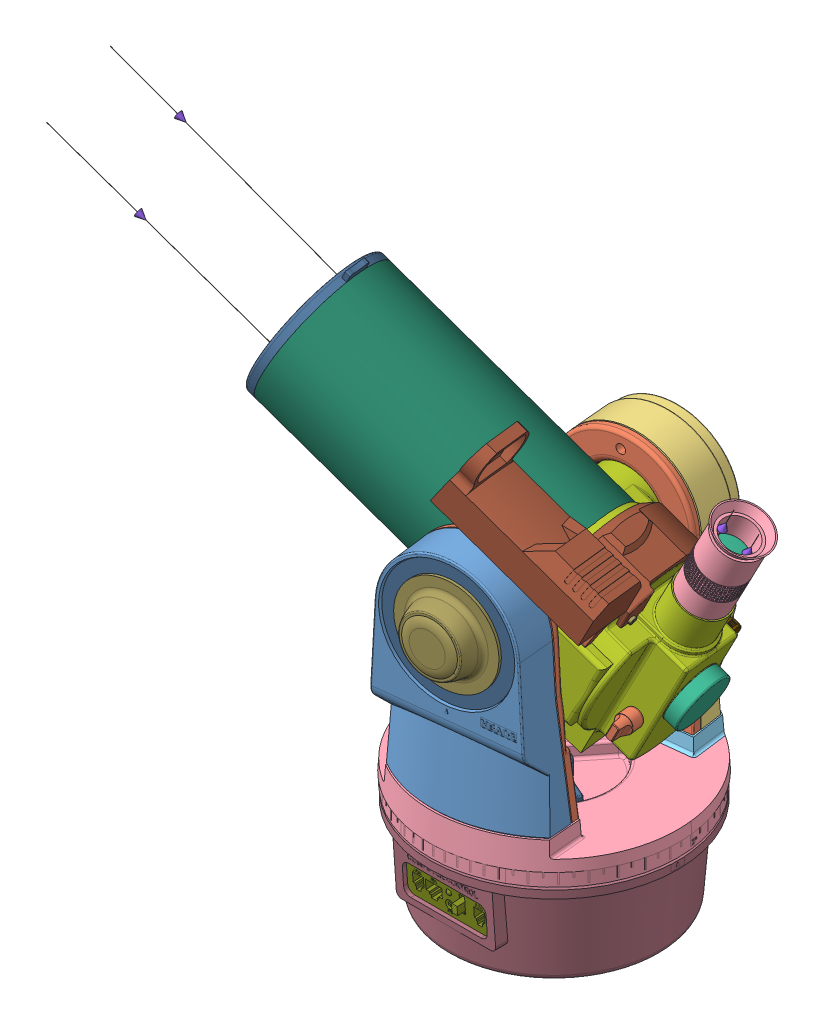
SolidWorks assembly meade, configuration Défaut. Lengths in mm.
Overall size (480.47 493.64 231.58).
168 component instances, 89 part files, 11 mates.
Components (placement in the parent):
- fourche-1: fourche [Défaut] at (-637.6539 13.0791 484.13) x (0.045417 -0.017413 0.998816) z (-0.998966 0.001172 0.045444) size (198.85 238.33 188.61)
  - branche equilibrage-1: branche equilibrage [Défaut] at (-444.0293 45.9192 -837.0232) x (0.999848 0.017413 0.00001) z (0.00001 -0.001172 0.999999) size (42.16 177.75 110.07)
  - Plaque carter équilibrage-1: Plaque carter équilibrage [Défaut] at (-443.0317 45.9366 -837.0903) x (0.999848 0.017413 0.00001) z (0.00001 -0.001172 0.999999) size (27.56 165.18 109.18)
  - Plaque carter équilibrage-2: Plaque carter équilibrage [Défaut] at (-468.0617 45.0668 -480.7137) x (-0.999848 -0.017413 -0.00001) z (-0.00001 0.001172 -0.999999) size (27.56 165.18 109.18)
  - branche motorisée-1: branche motorisée [Défaut] at (-441.716 45.9434 -837.1795) x (0.999848 0.017413 0.00001) z (0.00001 -0.001172 0.999999) size (49.59 177.72 110.04)
  - PIED DE fourche-1: PIED DE fourche [Défaut] at (-454.4692 -14.4541 -658.8869) x (0.999848 0.017413 0.00001) z (0.00001 -0.001172 0.999999) size (191.94 35.1 188.57)
    - Pied de fourche-1: Pied de fourche [Défaut] at (12.1809 59.9857 -178.2534) size (191.94 35.1 188.57)
    - Pied de fourche1-1: Pied de fourche1 [Défaut] at (-12.1809 59.9857 178.0188) x (-1 0 0) z (0 0 -1) size (54.8 35.1 115.86)
  - rondelle vis m8_50-1: rondelle vis m8_50 [Défaut] at (-454.2843 -25.0712 -659.0167) x (0.997592 0.017452 -0.067129) z (0.017413 -0.999848 -0.001172) size (26.8 26.16 7)
  - VisHM8_50-1: VisHM8_50 [Défaut] at (-454.3818 -19.4721 -659.0102) x (0.997592 0.017452 -0.067129) z (0.017413 -0.999848 -0.001172) size (12.6 14.55 55.47)
  - limiteur de couple embase-1: limiteur de couple embase [Défaut] at (-453.5008 -70.0544 -659.0694) x (0.06714 0 0.997744) z (-0.997592 -0.017452 0.067129) size (25.3 5 25.3)
  - Roue à denture hélicoïdale m=0,5 Z=60-1: Roue à denture hélicoïdale m=0,5 Z=60 [Défaut] at (-453.6431 -61.8856 -659.0599) x (0.201032 0.002353 0.979582) z (-0.017413 0.999848 0.001172) size (31.07 31.07 6.34)
  - Levier de débrayage-1: Levier de débrayage [Défaut] at (-491.4971 43.1006 -833.8173) x (0.963244 0.01709 -0.268082) z (0.268062 0.003539 0.963395) size (36.12 10 38.96)
  - plateau-1: plateau [Défaut] at (-454.3861 -19.2221 -659.0099) x (-0.997592 -0.017452 0.067129) z (0.017413 -0.999848 -0.001172) size (170 170 47)
  - EcrouHM 20-2: EcrouHM 20 [Défaut] at (-453.9456 -44.5183 -659.0395) x (0.06714 0 0.997744) z (-0.017413 0.999848 0.001172) size (30 34.64 12)
  - motoreducteur fourche-1: motoreducteur fourche [Défaut] at (-542.1299 45.8782 -641.824) x (0.06714 0 0.997744) z (0.997592 0.017452 -0.067129) size (70.5 139.71 33.06)
    - rep. 01 pignon arbre moteur + disque-1: rep. 01 pignon arbre moteur + disque [Défaut] at (0 -0.36 0) size (19 10.8 19)
    - rep. 02-03 roue Z56-1: rep. 02-03 roue Z56 [Défaut] at (0.8779 -0.6486 0.8082) x (0.995701 0 0.092628) z (-0.092628 0 0.995701) size (28.76 10.95 28.76)
    - rep. 08-09 roue inter-1: rep. 08-09 roue inter [Défaut] at (-0.15 -0.2381 0) x (1 0 0) z (0 0 1) size (12.96 5.74 12.96)
    - rep. 06-07 roue inter-1: rep. 06-07 roue inter [Défaut] at (-0.15 -0.0981 0) x (1 0 0) z (0 0 1) size (13 5.74 13)
    - rep. 04-05 roue inter-1: rep. 04-05 roue inter [Défaut] at (-21.6079 -0.6386 5.1059) x (0.907401 0 -0.420265) z (0.420265 0 0.907401) size (13 5.74 13)
    - bati-1: bati [Défaut] at (103.3128 129.885 -87.3106) size (70.5 138.91 24)
      - Axe Rep19bis-1: Axe Rep19bis [Défaut] at (-92.1856 -130.245 98.2871) x (-0.137137 0 0.990552) z (-0.990552 0 -0.137137) size (3 14 3)
      - moteur-1: moteur [Défaut] at (-103.3128 -129.885 87.3106) size (18 46.5 24)
      - axe-1: axe [Défaut] at (-111.605 -120.0821 97.7106) x (0.934599 0 -0.355704) z (0 -1 0) size (3 3 39)
      - bati2-1: bati2 [Défaut] at (-77.4849 -277.8736 138.6581) x (1 0 0) z (0 0 -1) size (17.4 55.11 17.4)
        - rondelle alu-1: rondelle alu [Défaut] at (-55.9783 -35.2009 30.6529) size (17.4 2.5 17.4)
        - Rondelle M6_1-1: Rondelle M6_1 [Défaut] at (-55.9783 -35.2009 30.6529) size (16.67 2.55 16.67)
        - rondelle alu_1-1: rondelle alu_1 [Défaut] at (-55.9783 -35.2009 30.6529) size (17.4 2.5 17.4)
        - Entretoise_1-1: Entretoise_1 [Défaut] at (-55.9783 -35.2009 30.6529) size (16.5 6 16.5)
        - Entretoise-1: Entretoise [Défaut] at (-55.9783 -35.2009 30.6529) size (16.5 6 16.5)
        - Rondelle M6-1: Rondelle M6 [Défaut] at (-55.9783 -35.2009 30.6529) size (16.67 2.55 16.67)
        - rep. 16 Ecrou M6-1: rep. 16 Ecrou M6 [Défaut] at (18.5294 -120.4752 48.0628) x (-0.896454 0 -0.443136) z (-0.443136 0 0.896454) size (12.68 6 11.39)
      - corps1-1: corps1 [Défaut] at (-126.5989 -147.7633 97.7106) size (62.7 74.5 12)
      - corps2-1: corps2 [Défaut] at (-126.5989 -147.7633 85.7106) size (62.7 50 12) (hidden)
      - châpe en alu-1: châpe en alu [Défaut] at (-133.4632 -157.3984 87.2051) size (33.3 38 19.61)
    - vis-1: vis [Défaut] at (7.3554 -71.4832 9.6533) x (1 0 0) z (0 1 0) size (33.09 33.06 82.71)
      - Vis san fin m=0,5 - 1 filet(s)-2: Vis san fin m=0,5 - 1 filet(s) [Défaut] at (-0.6479 -0.6412 0.3804) x (0.7262 -0.687484 0) z (0 0 1) size (8.16 8.16 68.9)
      - rep12-4: rep12 [Défaut] at (-11.6724 36.0347 43.7266) x (0.537117 -0.843508 0) z (-0.843508 -0.537117 0) size (23.91 29.81 24)
    - engrenage-1: engrenage [Défaut] at (-45.9983 -125.8694 31.0757) x (-0.919401 0 0.393321) z (0.393321 0 0.919401) size (12.99 17.44 12.99)
      - rep.11SLDPRT-1: rep.11SLDPRT [Défaut] at (-64.557 -106.8565 -14.5787) size (9.52 16 9.52)
      - rep. yacine-1: rep. yacine [Défaut] at (-64.557 -106.8565 -14.5787) size (12.99 1.44 12.99)
    - Vis à tête cylindrique à six pans creux Chc M2,5 - 8-1: Vis à tête cylindrique à six pans creux Chc M2,5 - 8 [Défaut] at (6.7074 -20.6971 10.2945) x (0.636786 0 0.771041) z (0 -1 0) size (4.2 4.2 10.57)
    - joint 9 5 emb-1: joint 9 5 emb [Défaut] at (6.7074 -89.1506 10.2945) size (13.5 2 13.5)
    - joint 9 5 emb-2: joint 9 5 emb [Défaut] at (6.7074 -53.1506 10.2945) size (13.5 2 13.5)
  - Vis sans tête à six pans creux à bout cuvette M3 - 3-1: Vis sans tête à six pans creux à bout cuvette M3 - 3 [Réaliste] at (-445.1418 -17.1499 -659.6319) x (-0.019293 -0.859815 -0.51024) z (0.066624 -0.510307 0.857408) size (3.03 3.08 3.04)
  - Vis à tête cylindrique bombée cruciforme type H M3 - 10-1: Vis à tête cylindrique bombée cruciforme type H M3 - 10 [Filetage Réaliste] at (-521.841 56.7793 -695.504) x (-0.997592 -0.017452 0.067129) z (-0.0364 0.955572 -0.292501) size (12.58 5.6 5.6)
  - Vis à tête cylindrique bombée cruciforme type H M3 - 10-2: Vis à tête cylindrique bombée cruciforme type H M3 - 10 [Filetage Réaliste] at (-508.9533 16.8988 -611.179) x (-0.997592 -0.017452 0.067129) z (-0.040277 -0.642181 -0.765494) size (12.58 5.6 5.6)
  - Vis à tête cylindrique bombée cruciforme type H M3 - 10-3: Vis à tête cylindrique bombée cruciforme type H M3 - 10 [Filetage Réaliste] at (-514.8616 16.8988 -698.9804) x (-0.997592 -0.017452 0.067129) z (-0.068087 0.06176 -0.995766) size (12.58 5.6 5.6)
  - Vis à tête cylindrique bombée cruciforme type H M3 - 10-4: Vis à tête cylindrique bombée cruciforme type H M3 - 10 [Filetage Réaliste] at (-521.2936 154.7556 -654.4481) x (-0.997592 -0.017452 0.067129) z (-0.06714 0 -0.997744) size (12.58 5.6 5.6)
  - Vis à tête cylindrique bombée cruciforme type H M3 - 10-5: Vis à tête cylindrique bombée cruciforme type H M3 - 10 [Filetage Réaliste] at (-516.3356 56.7793 -613.689) x (-0.997592 -0.017452 0.067129) z (-0.06714 0 -0.997744) size (12.58 5.6 5.6)
  - Vis à tête cylindrique bombée cruciforme type H M3 - 10-7: Vis à tête cylindrique bombée cruciforme type H M3 - 10 [Filetage Réaliste] at (-393.6444 157.0051 -663.0973) x (0.997592 0.017452 -0.067129) z (0.06714 0 0.997744) size (12.58 5.6 5.6)
  - Vis à tête cylindrique bombée cruciforme type H M3 - 10-8: Vis à tête cylindrique bombée cruciforme type H M3 - 10 [Filetage Réaliste] at (-401.1787 18.9039 -706.6898) x (0.997592 0.017452 -0.067129) z (0.06714 0 0.997744) size (12.58 5.6 5.6)
  - Vis à tête cylindrique bombée cruciforme type H M3 - 10-10: Vis à tête cylindrique bombée cruciforme type H M3 - 10 [Filetage Réaliste] at (-395.1895 59.0113 -704.086) x (0.997592 0.017452 -0.067129) z (0.06714 0 0.997744) size (12.58 5.6 5.6)
  - Vis à tête cylindrique fendue CS M4 - 10-1: Vis à tête cylindrique fendue CS M4 - 10 [Défaut] at (-539.7157 125.5672 -628.3483) x (0.067415 -0.016315 0.997592) z (-0.997592 -0.017452 0.067129) size (7 7 10.62)
  - Vis à tête cylindrique fendue CS M4 - 10-2: Vis à tête cylindrique fendue CS M4 - 10 [Défaut] at (-538.2089 116.0774 -615.8713) x (0.067415 -0.016315 0.997592) z (-0.997592 -0.017452 0.067129) size (7 7 10.62)
  - Vis à tête cylindrique fendue CS M4 - 10-3: Vis à tête cylindrique fendue CS M4 - 10 [Défaut] at (-539.3849 106.5701 -628.3705) x (0.067415 -0.016315 0.997592) z (-0.997592 -0.017452 0.067129) size (7 7 10.62)
  - Vis à tête cylindrique bombée cruciforme type H M3 - 12-2: Vis à tête cylindrique bombée cruciforme type H M3 - 12 [Filetage Réaliste] at (-395.2704 18.9039 -618.8883) x (0.997592 0.017452 -0.067129) z (0.067129 0.000586 0.997744) size (14.59 5.6 5.6)
  - Vis à tête cylindrique bombée cruciforme type H M3 - 12-3: Vis à tête cylindrique bombée cruciforme type H M3 - 12 [Filetage Réaliste] at (-389.684 59.0113 -622.271) x (0.997592 0.017452 -0.067129) z (0.068185 -0.42423 0.902984) size (14.59 5.6 5.6)
  - Vis à tête cylindrique bombée cruciforme type H M3 - 25-1: Vis à tête cylindrique bombée cruciforme type H M3 - 25 [Filetage Réaliste] at (-516.5693 58.6063 -628.1014) x (-0.997592 -0.017452 0.067129) z (-0.067129 0.486457 -0.871122) size (32.61 5.6 5.6)
  - Vis à tête cylindrique bombée cruciforme type H M3 - 25-2: Vis à tête cylindrique bombée cruciforme type H M3 - 25 [Filetage Réaliste] at (-520.3322 72.7741 -680.3366) x (-0.997592 -0.017452 0.067129) z (-0.067129 0.486457 -0.871122) size (32.61 5.6 5.6)
  - Vis à tête cylindrique bombée cruciforme type H M3 - 25-3: Vis à tête cylindrique bombée cruciforme type H M3 - 25 [Filetage Réaliste] at (-519.8272 43.7786 -680.3706) x (-0.997592 -0.017452 0.067129) z (0.067053 0.00493 0.997737) size (32.61 5.6 5.6)
  - Vis à tête cylindrique bombée cruciforme type H M3 - 20-1: Vis à tête cylindrique bombée cruciforme type H M3 - 20 [Filetage Réaliste] at (-531.1265 -25.9655 -653.8459) x (-0.017413 0.999848 0.001172) z (0.998816 0.017342 0.045444) size (22.61 5.6 5.6)
  - Vis à tête cylindrique bombée cruciforme type H M3 - 20-2: Vis à tête cylindrique bombée cruciforme type H M3 - 20 [Filetage Réaliste] at (-512.8439 -25.695 -612.9812) x (-0.017413 0.999848 0.001172) z (0.998816 0.017342 0.045444) size (22.61 5.6 5.6)
  - Vis à tête cylindrique bombée cruciforme type H M3 - 20-3: Vis à tête cylindrique bombée cruciforme type H M3 - 20 [Filetage Réaliste] at (-517.7505 -25.6821 -696.841) x (-0.017413 0.999848 0.001172) z (0.998816 0.017342 0.045444) size (22.61 5.6 5.6)
  - Vis à tête cylindrique bombée cruciforme type H M3 - 20-4: Vis à tête cylindrique bombée cruciforme type H M3 - 20 [Filetage Réaliste] at (-395.7403 -23.5476 -705.0512) x (-0.017413 0.999848 0.001172) z (0.998816 0.017342 0.045444) size (22.61 5.6 5.6)
  - Vis à tête cylindrique bombée cruciforme type H M3 - 20-5: Vis à tête cylindrique bombée cruciforme type H M3 - 20 [Filetage Réaliste] at (-377.4577 -23.2771 -664.1865) x (-0.017413 0.999848 0.001172) z (0.998816 0.017342 0.045444) size (22.61 5.6 5.6)
  - Vis à tête cylindrique bombée cruciforme type H M3 - 20-6: Vis à tête cylindrique bombée cruciforme type H M3 - 20 [Filetage Réaliste] at (-390.8337 -23.5604 -621.1914) x (-0.017413 0.999848 0.001172) z (0.998816 0.017342 0.045444) size (22.61 5.6 5.6)
- tube-1: tube [Défaut] at (-30.0954 77.7985 3.4044) x (0.112402 0 0.993663) z (-0.888013 0.448711 0.100451) size (229.47 195.18 484.9)
  - Capuchon port photo-2: Capuchon port photo [Défaut] at (20.0265 52.1414 -183.8549) x (0.753442 -0.654583 0.06202) z (-0.29492 -0.252137 0.921656) size (39.95 39.82 23.78)
  - support objectif-2: support objectif [Défaut] at (0 67.5 -76) size (179.88 130.77 134.7)
  - Palier d'embrayage-2: Palier d'embrayage [Défaut] at (24.7034 252.6163 -72.3954) x (0.997744 -0.06714 0) z (-0.06714 -0.997744 0) size (14.91 34.8 28.76)
  - palier-2: palier [Défaut] at (-93.6662 67.5 0) x (1 0 0) z (0 -0.589029 0.808112) size (10.05 25.5 25.5)
  - Roue à denture hélicoïdale m=0,5 Z=60-3: Roue à denture hélicoïdale m=0,5 Z=60 [Défaut] at (-77.15 67.5 0) x (0 0.783284 -0.621664) z (1 0 0) size (31.07 31.07 6.34)
  - Plaque repérage angulaire-3: Plaque repérage angulaire [Défaut] at (-159.1429 162.8547 -174.0321) x (0.997744 -0.051519 0.043053) z (-0.06714 -0.765605 0.639798) size (6.77 89 88.85)
  - molette blocage vertical-2: molette blocage vertical [Défaut] at (25.2373 156.4775 -169.1848) x (0.997744 -0.051429 0.043161) z (-0.06714 -0.764265 0.641398) size (31.87 70 69.98)
  - molette blocage 2 vertical-2: molette blocage 2 vertical [Défaut] at (-32.8172 155.1442 169.8822) x (-0.997741 -0.051084 -0.043619) z (0.067172 -0.759198 -0.647384) size (27.85 70 69.98)
  - Plaque repérage angulaire-4: Plaque repérage angulaire [Défaut] at (151.5627 161.1167 174.9858) x (-0.997741 -0.051084 -0.043619) z (0.067172 -0.759198 -0.647384) size (6.77 89 88.85)
  - Embout fileté-2: Embout fileté [Défaut] at (31.1097 71.2083 -217.7977) x (0.995668 0.069272 0.06202) z (-0.030498 -0.386808 0.921656) size (96.08 90.33 41.21)
  - miroir-2: miroir [Défaut] at (1.5401 49.2079 -414.2886) x (0 -0.998075 0.06202) z (-0.383759 0.057271 0.921656) size (89.51 86.43 44.67)
  - tube-2: tube [Défaut] at (0 67.5 -53.7618) x (0 0 -1) z (1 0 0) size (225 100 100)
  - menisque-2: menisque [Défaut] at (-10.827 126.3859 145.8849) x (-0.376431 0.924349 0.062271) z (0.377105 0.091483 0.921641) size (110.67 106.16 46.27)
    - menisque-1: menisque [Défaut] at (-56.116 -127.6725 -342.9742) size (27.57 28.77 19.69)
    - Piece1-1: Piece1 [Défaut] at (-57.8098 16.1933 3.3103) x (0.972599 -0.230535 0.030091) z (-0.028457 0.010411 0.999541) size (92 86.87 40.19)
  - molette-2: molette [Défaut] at (16.1783 77.4199 -201.1536) x (0.997152 -0.042906 0.06202) z (-0.073715 -0.380942 0.921656) size (12.27 29.01 54.01)
  - Vis porte oculaire-2: Vis porte oculaire [Défaut] at (70.5773 71.9334 3.0696) x (0.833291 0.517003 -0.195792) z (-0.515568 0.854579 0.062325) size (15.46 8.19 13.39)
  - bouton miroir-3: bouton miroir [Défaut] at (118.3372 40.7094 -82.3) x (0.999979 -0.006557 0) z (0 0 1) size (83.58 43.34 43.14)
    - bouton miroir-1: bouton miroir [Défaut] at (-90.8002 18.3233 -120.2299) x (0.996615 -0.012919 0.081184) z (-0.081184 -0.309873 0.947306) size (41.27 12.61 13.28)
    - bouton miroir-2: bouton miroir [Défaut] at (-145.9581 -6.2943 -120.2299) x (-0.996615 0.012919 0.081184) z (0.081184 0.309873 0.947306) size (41.27 12.61 13.28)
    - petit miroir-1: petit miroir [Défaut] at (-118.5103 26.0141 2.75) x (0.999979 0.006557 0) z (0.004637 -0.707092 0.707107) size (30 26.01 35)
  - oculaire-2: oculaire [Défaut] at (0 149.5136 -0.7045) x (0 0 1) z (-1 0 0) size (38 81.5 38)
    - oculaire-1: oculaire [Défaut] at (-78.8455 -41.743 0) size (38 81.5 38)
    - lentille-1: lentille [Défaut] at (-81.1151 5.0064 0) x (0 -1 0) z (0 0 1) size (10.53 25 25)
      - lentille 1-1: lentille 1 [Défaut] at (-6.7507 2.2696 0) size (8.01 25 25)
      - lentille 2-1: lentille 2 [Défaut] at (-12.7507 2.2696 0) size (4.52 25 25)
    - lentille-2: lentille [Défaut] at (-76.963 10.0077 1.2678) x (0 1 0) z (-0.558618 0 0.829425) size (10.53 25 25)
      - lentille 1-1: lentille 1 [Défaut] at (-6.7507 2.2696 0) size (8.01 25 25)
      - lentille 2-1: lentille 2 [Défaut] at (-12.7507 2.2696 0) size (4.52 25 25)
  - faisceau2-2: faisceau2 [Défaut] at (0 78.827 -14.9477) x (0 0 -1) z (1 0 0) size (437.42 120.49 0.34)
  - fleche-13: fleche [Défaut] at (0 108.7031 110.8339) x (0 0 1) z (-0.886861 -0.462037 0) size (8 5.6 5.6)
  - fleche-14: fleche [Défaut] at (0 88.228 83.446) x (0 0.178036 -0.984024) z (1 -0.000403 -0.000073) size (8 5.6 5.6)
  - fleche-15: fleche [Défaut] at (0 75.6322 94.3005) x (0 0.005533 0.999985) z (0.072331 0.997365 -0.005519) size (8 5.6 5.6)
  - fleche-16: fleche [Défaut] at (0 108.7103 294.2676) x (0 0.017452 0.999848) z (-0.523715 0.851763 -0.014868) size (8 5.6 5.6)
  - fleche-17: fleche [Défaut] at (0 127.4306 -74.061) x (0 -0.974863 -0.222804) z (-0.735553 0.150943 -0.660438) size (8 5.6 5.6)
  - fleche-18: fleche [Défaut] at (0 183.519 -69.8214) x (0 -1 0) z (-0.316126 0 0.948717) size (8 5.6 5.6)
  - faisceau1-2: faisceau1 [Défaut] at (0 -20.7845 -6.8996) x (0 0 -1) z (1 0 0) size (447.26 167.74 0.41)
  - fleche-19: fleche [Défaut] at (0 30.6251 284.852) x (0 0 1) z (-0.426184 0.904636 0) size (8 5.6 5.6)
  - fleche-20: fleche [Défaut] at (0 27.6512 105.4051) x (0 0 1) z (-0.740163 -0.672427 0) size (8 5.6 5.6)
  - fleche-21: fleche [Défaut] at (0 46.7601 79.6116) x (0 -0.171906 -0.985113) z (0.984293 0.173915 -0.030349) size (8 5.6 5.6)
  - fleche-22: fleche [Défaut] at (0 59.5724 94.0494) x (0 -0.005145 0.999987) z (-0.101559 -0.994816 -0.005119) size (8 5.6 5.6)
  - fleche-23: fleche [Défaut] at (0 127.1897 -84.7907) x (0 -0.982309 0.187268) z (-0.405585 0.171174 0.897887) size (8 5.6 5.6)
  - fleche-24: fleche [Défaut] at (0 183.4575 -88.3366) x (0 -1 0) z (-0.976187 0 0.216931) size (8 5.6 5.6)
  - cache-2: cache [Défaut] at (0 67.5 174.5) x (0 0 -1) z (1 0 0) size (10 111 100)
  - Module LNT-2: Module LNT [Défaut] at (0 67.5 -16) x (0.999806 -0.019718 0) z (0 0 1) size (140.9 99.11 110)
  - Vis à tête cylindrique fendue CS M3 - 10-1: Vis à tête cylindrique fendue CS M3 - 10 [Défaut] at (27 106.7707 -61.5) size (5.5 5.5 12.01)
  - Pièce1^tube-1: Pièce1^tube [Défaut] at origin (virtual)
- CARTER EMBASE-2: CARTER EMBASE [Défaut] at (-38.5593 -33.7526 0) x (-1 0 0) z (0 0 -1) size (208.81 81 208.82)
  - Carter embase-1: Carter embase [Défaut] at (-38.5593 34.3526 0) size (182.1 77.5 182)
  - palier-1: palier [Défaut] at (-38.7022 18.1339 0.128) x (-0.744983 0 0.667084) z (0.667084 0 0.744983) size (45.68 15.3 45.68)
    - palier alu-1: palier alu [Défaut] at (-0.1919 7.7813 0) size (40 13.5 40)
    - palier axial-1: palier axial [Défaut] at (-0.1919 -6.6187 0) size (33 6.3 33)
    - palier axial-2: palier axial [Défaut] at (-0.1919 8.6813 0) x (-0.837169 0 -0.546944) z (-0.546944 0 0.837169) size (33 6.3 33)
  - plaque branchement-1: plaque branchement [Défaut] at (-38.5593 -18.7385 -76.5024) x (1 0 0) z (0 0.068841 0.997628) size (62.31 43.19 20.2)
  - carter couvercle-1: carter couvercle [Défaut] at (-38.5593 -43.1474 0) x (0 0 1) z (-1 0 0) size (145 23 145)
  - anneau guide-1: anneau guide [Défaut] at (-38.5593 19.8526 0) x (-0.683843 0 0.729629) z (0 1 0) size (46.6 56.5 4.2)
  - support palier-1: support palier [Défaut] at (-38.5593 58.1532 0) x (0.258819 0 -0.965926) z (0.965926 0 0.258819) size (170.5 70.67 170.49)
  - reducteur embase-1: reducteur embase [Défaut] at (-74.9499 2.4826 -18.0358) x (0 0 1) z (0 -1 0) size (101.77 85.1 39.66)
    - rep. 01 pignon arbre moteur + disque-1: rep. 01 pignon arbre moteur + disque [Défaut] at (0.9543 -1.36 18.0797) x (0.78085 0 0.624719) z (-0.624719 0 0.78085) size (19 10.8 19)
    - rep. 02-03 roue Z56-1: rep. 02-03 roue Z56 [Défaut] at (-12.7174 -0.5 -2.1104) x (0.531735 0 -0.846911) z (0.846911 0 0.531735) size (28.76 10.95 28.76)
    - rep. 08-09 roue inter-1: rep. 08-09 roue inter [Défaut] at (-2.3943 -0.3381 0.4364) x (0.975998 0 -0.217777) z (0.217777 0 0.975998) size (12.96 5.74 12.96)
    - rep. 06-07 roue inter-1: rep. 06-07 roue inter [Défaut] at (-3.1771 0.3019 0.7148) x (0.955582 0 -0.294727) z (0.294727 0 0.955582) size (13 5.74 13)
    - roue rep 12 (petite folle)-1: roue rep 12 (petite folle) [Défaut] at (0.2679 -0.4 -0.3808) x (0.999222 0 0.039446) z (-0.039446 0 0.999222) size (13 3.24 13)
    - rep. 04-05 roue inter-1: rep. 04-05 roue inter [Défaut] at (2.2907 -0.16 -1.8606) x (0.977065 0 0.21294) z (-0.21294 0 0.977065) size (13 5.74 13)
    - bati emb-1: bati emb [Défaut] at (103.3128 129.885 -87.3106) size (101.77 84.35 25.96)
      - coque droite emb-1: coque droite emb [Défaut] at (-103.3128 -129.885 87.3106) size (93.29 54 12.58)
      - Axe Rep19bis emb-1: Axe Rep19bis emb [Défaut] at (-103.9752 -130.143 87.3656) x (0.998781 0 -0.049366) z (0.049366 0 0.998781) size (3 15.3 3)
      - Axe Rep20.bis emb-1: Axe Rep20.bis emb [Défaut] at (-97.8983 -130.0094 79.9317) x (0.927514 0 0.373788) z (-0.373788 0 0.927514) size (3 22 3)
      - coque gauche emb-1: coque gauche emb [Défaut] at (-103.3128 -129.885 87.3106) size (94.76 55 11.51)
      - axe emb-1: axe emb [Défaut] at (-111.605 -119.0221 97.7106) x (0.824702 0 -0.565567) z (0 -1 0) size (3 3 15)
      - Axe Rep19bis emb-2: Axe Rep19bis emb [Défaut] at (-101.4828 -129.945 90.8669) x (0.715658 0 -0.698451) z (0.698451 0 0.715658) size (3 15.3 3)
      - moteur-2: moteur [Défaut] at (-103.3128 -129.885 87.3106) size (18 46.5 24)
      - châpe en alu emb-2: châpe en alu emb [Défaut] at (-103.4628 -123.4884 87.3106) size (32 38 21)
      - Entretoise emb-3: Entretoise emb [Défaut] at (-100.6729 -123.5884 80.7498) x (0.982912 0 0.184074) z (-0.184074 0 0.982912) size (17.65 5.7 17.65)
      - rondelle alu emb-3: rondelle alu emb [Défaut] at (-90.9589 -123.8884 68.1548) x (0.821605 0 0.570058) z (-0.570058 0 0.821605) size (17.4 2.65 17.4)
      - rep. 16 Ecrou M6 emb-2: rep. 16 Ecrou M6 emb [Défaut] at (-102.7157 -122.485 84.9564) x (0.99792 0 0.06446) z (-0.06446 0 0.99792) size (12.68 6 11.39)
      - Rondelle M6 emb-2: Rondelle M6 emb [Défaut] at (-94.2052 -123.7384 71.161) x (0.88187 0 0.471493) z (-0.471493 0 0.88187) size (16 1.8 16)
      - joint 9 5 emb-3: joint 9 5 emb [Défaut] at (-66.605 -149.1255 97.7106) size (13.5 2 13.5)
      - joint 9 5 emb-4: joint 9 5 emb [Défaut] at (-66.605 -183.1255 97.7106) x (0.837169 0 0.546944) z (0.546944 0 -0.837169) size (13.5 2 13.5)
      - rondelle alu emb-4: rondelle alu emb [Défaut] at (-91.5165 -167.7384 68.6232) x (0.832295 0 0.554332) z (-0.554332 0 0.832295) size (17.4 2.65 17.4)
      - Entretoise emb-4: Entretoise emb [Défaut] at (-30.2975 -208.6627 109.115) x (-0.835834 0 -0.548983) z (-0.548983 0 0.835834) size (17.65 5.7 17.65)
      - Rondelle M6 emb-3: Rondelle M6 emb [Défaut] at (-29.9622 -208.5127 109.2274) x (-0.837169 0 -0.546944) z (-0.546944 0 0.837169) size (16 1.8 16)
      - Vis à tête cylindrique bombée cruciforme type H M3 - 12-1: Vis à tête cylindrique bombée cruciforme type H M3 - 12 [Filetage Réaliste] at (-110.205 -142.8221 109.7106) x (0 0 -1) z (1 0 0) size (14.59 5.6 5.6)
      - Vis à tête cylindrique bombée cruciforme type H M3 - 12-2: Vis à tête cylindrique bombée cruciforme type H M3 - 12 [Filetage Réaliste] at (-93.3519 -120.1721 111.5106) x (0 0 -1) z (-0.592827 0.80533 0) size (14.59 5.6 5.6)
    - vis emb-1: vis emb [Défaut] at (37.3558 -36.1406 9.7588) x (1 0 0) z (0 1 0) size (25.74 25.82 76.16)
      - Vis san fin m=0,5 - 1 filet(s) emb-1: Vis san fin m=0,5 - 1 filet(s) emb [Défaut] at (-0.6479 -0.6412 0) size (8.16 8.16 68.9)
      - rep12 emb-3: rep12 emb [Défaut] at (-38.2155 6.7975 36.7974) x (0.996839 0.079451 0) z (0.079451 -0.996839 0) size (23.91 23.8 24)
    - engrenage-1: engrenage [Défaut] at (64.1683 106.4565 3.5924) x (0.967334 0 -0.253504) z (0.253504 0 0.967334) size (12.99 17.44 12.99)
      - rep.11SLDPRT-1: rep.11SLDPRT [Défaut] at (-64.557 -106.8565 -14.5787) size (9.52 16 9.52)
      - rep. yacine-1: rep. yacine [Défaut] at (-64.557 -106.8565 -14.5787) size (12.99 1.44 12.99)
    - Vis à tête cylindrique à six pans creux Chc M2,5 - 8-1: Vis à tête cylindrique à six pans creux Chc M2,5 - 8 [Défaut] at (36.7078 7.7163 10.4) x (1 0 0) z (0 -1 0) size (4.2 4.2 10.57)
  - Vis à tête fraisée FS M5 - 16-1: Vis à tête fraisée FS M5 - 16 [Défaut] at (-102.5593 -40.456 0) x (-1 0 0) z (0 1 0) size (10.32 10.4 16)
  - Vis à tête fraisée FS M5 - 16-2: Vis à tête fraisée FS M5 - 16 [Défaut] at (-6.5593 -40.456 55.4256) x (0.5 0 0.866025) z (0 1 0) size (10.32 10.4 16)
  - Vis à tête fraisée FS M5 - 16-3: Vis à tête fraisée FS M5 - 16 [Défaut] at (-6.5593 -40.456 -55.4256) x (0.5 0 -0.866025) z (0 1 0) size (10.32 10.4 16)
  - Vis à tête cylindrique bombée cruciforme type H M3 - 12-1: Vis à tête cylindrique bombée cruciforme type H M3 - 12 [Filetage Réaliste] at (-58.5127 -18.1174 -56.178) x (0 1 0) z (0 0 1) size (14.59 5.6 5.6)
  - Vis à tête cylindrique bombée cruciforme type H M3 - 12-2: Vis à tête cylindrique bombée cruciforme type H M3 - 12 [Filetage Réaliste] at (-89.2627 -18.7174 28.322) x (0 1 0) z (0 0 1) size (14.59 5.6 5.6)
  - Vis à tête cylindrique fendue CS M4 - 10-1: Vis à tête cylindrique fendue CS M4 - 10 [Défaut] at (-38.4593 -1.6174 37.562) x (1 0 0) z (0 1 0) size (7 7 10.62)
  - Vis à tête cylindrique fendue CS M4 - 10-2: Vis à tête cylindrique fendue CS M4 - 10 [Défaut] at (-31.0593 -0.5174 24.912) x (1 0 0) z (0 1 0) size (7 7 10.62)
  - Vis à tête cylindrique fendue CS M4 - 10-3: Vis à tête cylindrique fendue CS M4 - 10 [Défaut] at (-45.8593 -0.5174 24.912) x (1 0 0) z (0 1 0) size (7 7 10.62)
Mates (geometry in assembly coordinates):
- Coïncidente76: coincident: line of fourche-1/Roue à denture hélicoïdale m=0,5 Z=60-1 through (0 -90.27 0) axis (0 1 0); plane of ?
- Coïncidente71: coincident anti-aligned: plane of fourche-1/branche motorisée-1; plane of ? through (-85.4162 148.1836 8.0295) normal (-1 0 0)
- Coaxiale7: concentric anti-aligned: cylinder of ? through (-86.4662 138.2317 0.0594) axis (-1 0 0) radius 2.25; circle of fourche-1/Plaque carter équilibrage-2
- Coïncidente51: coincident: point of ?; plane of fourche-1/Plaque carter équilibrage-1 through (24.4187 65.7424 0) normal (0 0 1)
- Coïncidente80: coincident aligned: plane of ? through (0 140.7631 -55.645) normal (1 0 0); plane of assembly through (0 0 0) normal (1 0 0)
- Coïncidente84: coincident anti-aligned: plane of fourche-1/branche motorisée-1 through (-9.6003 138.1217 -84.875) normal (0.112402 0 0.993663); plane of tube-1/palier-2 through (-11.6754 150.6995 -84.6403) normal (-0.112402 0 -0.993663)
- Coaxiale10: concentric anti-aligned: cylinder of fourche-1/branche motorisée-1 through (-9.6003 138.1217 -84.875) axis (0.112402 0 0.993663) radius 12; cylinder of tube-1/palier-2 through (-10.5276 138.1217 -93.0727) axis (-0.112402 0 -0.993663) radius 12
- Coïncidente91: coincident anti-aligned: plane of CARTER EMBASE-2 through (-38.5593 -33.7526 0) normal (0 0 -1); plane of assembly through (0 0 0) normal (0 0 1)
- Coaxiale14: concentric aligned: cylinder of fourche-1/plateau-1 through (0 1 0) axis (0 1 0) radius 11; cylinder of CARTER EMBASE-2/palier-1/palier axial-1 through (0 -9 0) axis (0 1 0) radius 11.2
- Coïncidente92: coincident anti-aligned: plane of fourche-1/plateau-1 through (15.6155 -9 -32.437) normal (0 -1 0); plane of CARTER EMBASE-2/palier-1/palier axial-1 through (-12.2922 -9 11.0069) normal (0 1 0)
- Coïncidente93: coincident anti-aligned: plane of CARTER EMBASE-2/palier-1/palier axial-2 through (4.2705 -24.3 -15.9378) normal (0 -1 0); plane of fourche-1/EcrouHM 20-2 through (17.8252 -24.3 24.1301) normal (0 1 0)
